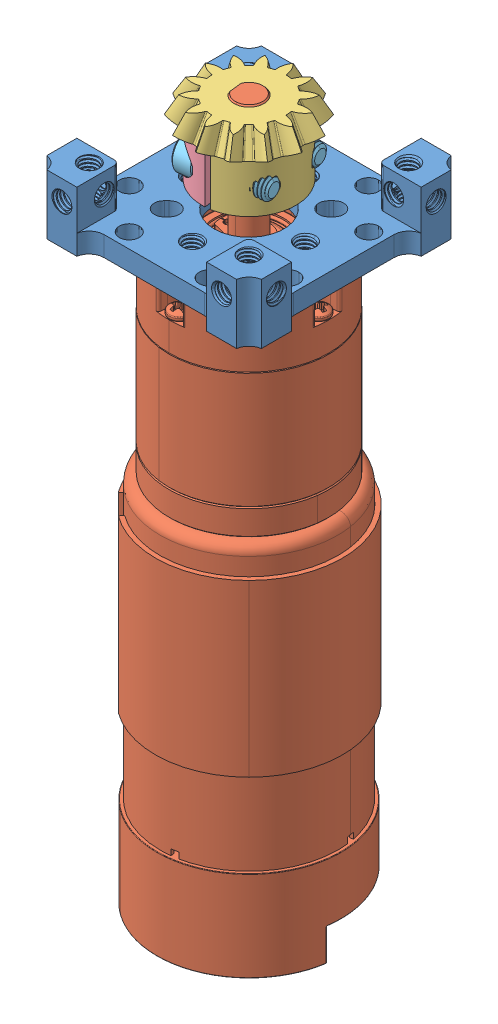
SolidWorks assembly 435 RPM Motor In Quad Block with Bevel, configuration Default. Lengths in mm.
Overall size (43.01 141.28 43.01).
7 component instances, 5 part files, 6 mates.
Components (placement in the parent):
- Quad Block.step-1: Quad Block.step [Default] at origin size (43.01 12.01 43.01)
- 435 RPM Motor.step-1: 435 RPM Motor.step [Default] x (1 0 0) z (0 1 0) size (37.51 37.5 140.7)
- Bevel.STEP-1: Bevel.STEP [Default] at (-11.884 6.8884 -1.3621) x (0 1 0) z (0.10797 0 0.994154) size (15.33 23.91 24.42)
  - 2306-0006-0014.STEP-1: 2306-0006-0014.STEP [Default] at (11.7425 -11.6675 2.6373) size (15.33 23.91 24.42)
  - 2306-0006-0014 clamp.STEP-1: 2306-0006-0014 clamp.STEP [Default] at (11.742 -11.6675 2.6373) size (9.55 8.86 18.69)
  - 2800-0004-0012_90128A207.STEP-1: 2800-0004-0012_90128A207.STEP [Default] at (7.1337 -20.4175 7.8873) x (0.998516 0 -0.054455) z (0 -1 0) size (7 7 16.01)
  - 2800-0004-0012_90128A207.STEP-2: 2800-0004-0012_90128A207.STEP [Default] at (7.1337 -20.4175 -2.6127) x (1 0 0) z (0 -1 0) size (7 7 16.01)
Mates (geometry in assembly coordinates):
- Coincident1: coincident: plane of Quad Block.step-1 through (0 0 0) normal (0 -1 0); plane of 435 RPM Motor.step-1 through (0 0 0) normal (0 1 0)
- Concentric2: concentric: circle of Quad Block.step-1; circle of 435 RPM Motor.step-1
- Coincident2: coincident: circle of Quad Block.step-1; circle of 435 RPM Motor.step-1
- Concentric3: concentric: cylinder of 435 RPM Motor.step-1 through (0 24 0) axis (0 -1 0) radius 3; cylinder of Bevel.STEP-1/2306-0006-0014.STEP-1 through (0 1.1458 0) axis (0 1 0) radius 3
- Parallel2: parallel: line of 435 RPM Motor.step-1 through (-2.3008 24 1.5062) axis (-0.10797 0 -0.994154); line of Bevel.STEP-1/2306-0006-0014.STEP-1 through (-2.2832 15.6457 1.946) axis (-0.10797 0 -0.994154)
- Coincident10: coincident: circle of 435 RPM Motor.step-1; circle of Bevel.STEP-1/2306-0006-0014.STEP-1
